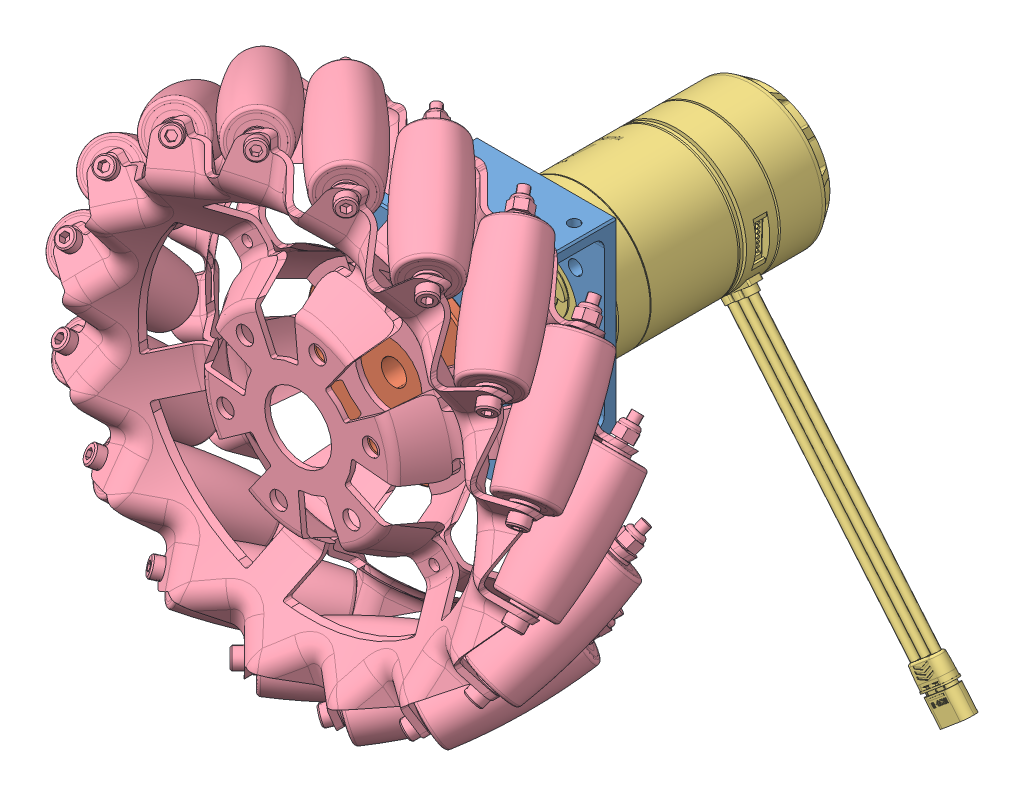
SolidWorks assembly 麦轮电机总装右, configuration 默认. Lengths in mm.
Overall size (225.34 230.35 154.77).
5 component instances, 4 part files, 3 mates.
Components (placement in the parent):
- 3508电机-1: 3508电机 [Default] at (20.407 2.6404 90.2458) size (124.33 157.68 116.9)
  - 电机座Z80123-1: 电机座Z80123 [默认] at (-77.6885 26.4734 96.0875) size (42 55.4 32)
  - 电机连轴Z80123-1: 电机连轴Z80123 [默认] at (-77.6885 26.4734 125.8875) x (0.707107 -0.707107 0) z (0.707107 0.707107 0) size (55 37.5 55)
  - M3508直流无刷减速电机-2: M3508直流无刷减速电机 [默认] at (-69.0293 10.2886 -6.3535) x (0.923508 0.383579 0) z (0 0 1) size (63.71 141 98.4)
- 麦轮镂空（右）-1: 麦轮镂空（右） [默认] at (-150.2658 -73.4679 151.1394) x (-0.707107 0.707107 0) z (0.707107 0.707107 0) size (182.09 47.13 182.09)
Mates (geometry in assembly coordinates):
- 同心1: concentric aligned: cylinder of 3508电机-1/电机连轴Z80123-1 through (-57.2815 29.1138 216.1333) axis (0 0 -1) radius 3.75; cylinder of 麦轮镂空（右）-1 through (-57.2815 29.1138 244.895) axis (0 0 -1) radius 10
- 同心2: concentric aligned: cylinder of 3508电机-1/电机连轴Z80123-1 through (-73.1914 45.0237 205.1333) axis (0 0 1) radius 2.6; cylinder of 麦轮镂空（右）-1 through (-73.1914 45.0237 242.9723) axis (0 0 1) radius 2.6
- 重合1: coincident anti-aligned: plane of 3508电机-1/电机连轴Z80123-1 through (-57.2815 29.1138 216.1333) normal (0 0 1); plane of 麦轮镂空（右）-1 through (-52.8331 -16.0519 216.1333) normal (0 0 -1)
